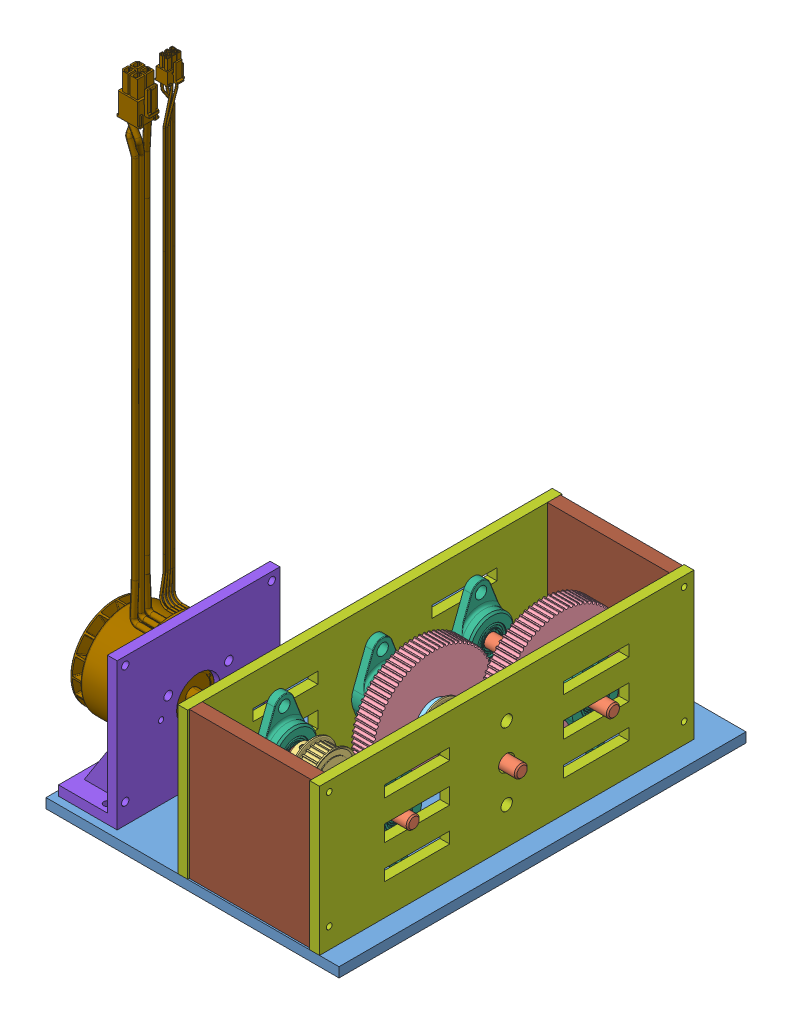
SolidWorks assembly Assembly, configuration Default. Lengths in mm.
Overall size (191.99 374.93 250).
22 component instances, 11 part files, 55 mates.
Components (placement in the parent):
- Base plate-1: Base plate [Default] at (107.5559 97.829 204.5167) size (180 6 250)
- 1265K67_Rotary Shaft-1: 1265K67_Rotary Shaft [1265K67] at (-105.0192 148.829 214.5167) x (0 -0.466171 -0.884694) z (1 0 0) size (8 8 100)
- 1265K67_Rotary Shaft-2: 1265K67_Rotary Shaft [1265K67] at (-110.9869 148.829 274.9267) x (0 -0.994866 -0.101198) z (1 0 0) size (8 8 100)
- 1265K67_Rotary Shaft-3: 1265K67_Rotary Shaft [1265K67] at (-108.8223 148.829 154.1067) x (0 0.698685 0.715429) z (1 0 0) size (8 8 100)
- 26toothpulley.stp-1: 26toothpulley.stp [Default] at (126.6866 148.829 274.9267) x (0 0.982193 0.187876) z (-1 0 0) size (28.1 28.1 20.6)
- 26toothpulley.stp-2: 26toothpulley.stp [Default] at (157.7866 148.829 214.5167) x (0 0.532948 0.846148) z (1 0 0) size (28.1 28.1 20.6)
- 80toothpulley.stp-1: 80toothpulley.stp [Default] at (146.2866 148.829 154.1067) x (0 0.075544 -0.997142) z (-1 0 0) size (75.56 75.56 22.2)
- 80toothpulley.stp-2: 80toothpulley.stp [Default] at (127.9866 148.829 214.5167) x (0 -0.170315 0.98539) z (-1 0 0) size (75.56 75.56 22.2)
- 94630A112_Steel Oversized Washer-1: 94630A112_Steel Oversized Washer [94630A112] at (144.9866 148.829 214.5167) x (0 -0.091283 0.995825) z (-1 0 0) size (23 23 4.3)
- 2820T42_Dry-Running Mounted Sleeve Bearing (1)-1: 2820T42_Dry-Running Mounted Sleeve Bearing (1) [2820T42] at (173.8059 148.829 154.1067) x (0 1 0) z (-1 0 0) size (57 28.5 11.75)
- 2820T42_Dry-Running Mounted Sleeve Bearing (1)-2: 2820T42_Dry-Running Mounted Sleeve Bearing (1) [2820T42] at (110.3059 148.829 274.9267) x (0 -1 0) z (1 0 0) size (57 28.5 11.75)
- 2820T42_Dry-Running Mounted Sleeve Bearing (1)-3: 2820T42_Dry-Running Mounted Sleeve Bearing (1) [2820T42] at (110.3059 148.829 214.5167) x (0 1 0) z (1 0 0) size (57 28.5 11.75)
- 2820T42_Dry-Running Mounted Sleeve Bearing (1)-4: 2820T42_Dry-Running Mounted Sleeve Bearing (1) [2820T42] at (173.8059 148.829 214.5167) x (0 1 0) z (-1 0 0) size (57 28.5 11.75)
- 2820T42_Dry-Running Mounted Sleeve Bearing (1)-5: 2820T42_Dry-Running Mounted Sleeve Bearing (1) [2820T42] at (110.3059 148.829 154.1067) x (0 -1 0) z (1 0 0) size (57 28.5 11.75)
- 2820T42_Dry-Running Mounted Sleeve Bearing (1)-6: 2820T42_Dry-Running Mounted Sleeve Bearing (1) [2820T42] at (173.8059 148.829 274.9267) x (0 1 0) z (-1 0 0) size (57 28.5 11.75)
- Shaft_and_Bearing_plate-1: Shaft_and_Bearing_plate [Default] at (104.5559 148.829 214.5167) x (0 0 1) z (0 -1 0) size (230 6 90)
- Shaft_and_Bearing_plate-2: Shaft_and_Bearing_plate [Default] at (179.5559 148.829 214.5167) x (0 0 -1) z (0 -1 0) size (230 6 90)
- motor_plate-1: motor_plate [Default] at (56.653 148.829 274.9267) x (0 0 -1) z (0 1 0) size (100 36 90)
- EC60fl-200W-V2.stp-1: EC60fl-200W-V2.stp [Default] at (73.753 148.829 274.9267) x (-1 0 0) z (0 0 1) size (68.19 353.93 60)
- 2463K28_Clamping Precision Flexible Shaft Coupling-1: 2463K28_Clamping Precision Flexible Shaft Coupling [2463K28] at (80.6759 148.829 274.9267) x (0 -0.924225 -0.381849) z (1 0 0) size (26.29 26.14 30)
- side_plate-1: side_plate [Default] at (142.0559 148.829 100.5167) x (1 0 0) z (0 -1 0) size (75 8 90)
- side_plate-2: side_plate [Default] at (142.0559 148.829 320.5167) x (1 0 0) z (0 -1 0) size (75 8 90)
Mates (geometry in assembly coordinates):
- Concentric1: concentric: cylinder of 1265K67_Rotary Shaft-2 through (189.0131 148.829 274.9267) axis (-1 0 0) radius 4; cylinder of 26toothpulley.stp-1 through (118.4966 148.829 274.9267) axis (1 0 0) radius 3
- Concentric2: concentric: cylinder of 1265K67_Rotary Shaft-1 through (194.9808 148.829 214.5167) axis (-1 0 0) radius 4; cylinder of 80toothpulley.stp-2 through (118.0116 148.829 214.5167) axis (1 0 0) radius 4
- Concentric3: concentric anti-aligned: cylinder of 1265K67_Rotary Shaft-1 through (194.9808 148.829 214.5167) axis (-1 0 0) radius 4; cylinder of 94630A112_Steel Oversized Washer-1 through (140.6866 148.829 214.5167) axis (1 0 0) radius 4.2
- Concentric4: concentric aligned: cylinder of 1265K67_Rotary Shaft-1 through (194.9808 148.829 214.5167) axis (-1 0 0) radius 4; cylinder of 26toothpulley.stp-2 through (165.9766 148.829 214.5167) axis (-1 0 0) radius 3
- Coincident2: coincident anti-aligned: plane of 80toothpulley.stp-2 through (140.6866 148.829 214.5167) normal (1 0 0); circle of 94630A112_Steel Oversized Washer-1
- Coincident3: coincident anti-aligned: plane of 26toothpulley.stp-2 through (144.9866 148.829 214.5167) normal (-1 0 0); plane of 94630A112_Steel Oversized Washer-1 through (144.9866 148.829 214.5167) normal (1 0 0)
- Concentric6: concentric anti-aligned: cylinder of 1265K67_Rotary Shaft-3 through (191.1777 148.829 154.1067) axis (-1 0 0) radius 4; cylinder of 80toothpulley.stp-1 through (136.3116 148.829 154.1067) axis (1 0 0) radius 4
- Concentric7: concentric: cylinder of 1265K67_Rotary Shaft-3 through (191.1777 148.829 154.1067) axis (-1 0 0) radius 4; cylinder of 2820T42_Dry-Running Mounted Sleeve Bearing (1)-1 through (168.0559 148.829 154.1067) axis (-1 0 0) radius 3.995
- Concentric8: concentric: cylinder of 1265K67_Rotary Shaft-3 through (191.1777 148.829 154.1067) axis (-1 0 0) radius 4; cylinder of 2820T42_Dry-Running Mounted Sleeve Bearing (1)-5 through (116.0559 148.829 154.1067) axis (1 0 0) radius 3.995
- Concentric9: concentric: cylinder of 1265K67_Rotary Shaft-1 through (194.9808 148.829 214.5167) axis (-1 0 0) radius 4; cylinder of 2820T42_Dry-Running Mounted Sleeve Bearing (1)-4 through (168.0559 148.829 214.5167) axis (-1 0 0) radius 3.995
- Concentric10: concentric anti-aligned: cylinder of 1265K67_Rotary Shaft-1 through (194.9808 148.829 214.5167) axis (-1 0 0) radius 4; cylinder of 2820T42_Dry-Running Mounted Sleeve Bearing (1)-3 through (116.0559 148.829 214.5167) axis (1 0 0) radius 3.995
- Concentric11: concentric: cylinder of 1265K67_Rotary Shaft-2 through (189.0131 148.829 274.9267) axis (-1 0 0) radius 4; cylinder of 2820T42_Dry-Running Mounted Sleeve Bearing (1)-6 through (168.0559 148.829 274.9267) axis (-1 0 0) radius 3.995
- Concentric12: concentric: cylinder of 1265K67_Rotary Shaft-2 through (189.0131 148.829 274.9267) axis (-1 0 0) radius 4; cylinder of 2820T42_Dry-Running Mounted Sleeve Bearing (1)-2 through (116.0559 148.829 274.9267) axis (1 0 0) radius 3.995
- Concentric13: concentric: cylinder of 1265K67_Rotary Shaft-1 through (194.9808 148.829 214.5167) axis (-1 0 0) radius 4; cylinder of Shaft_and_Bearing_plate-1 through (98.5559 148.829 214.5167) axis (1 0 0) radius 5
- Coincident4: coincident: plane of Base plate-1 through (107.5559 103.829 204.5167) normal (0 1 0); plane of Shaft_and_Bearing_plate-1 through (98.5559 103.829 99.5167) normal (0 -1 0)
- Coincident5: coincident: plane of Base plate-1 through (107.5559 103.829 204.5167) normal (0 1 0); plane of Shaft_and_Bearing_plate-2 through (185.5559 103.829 329.5167) normal (0 -1 0)
- Parallel1: parallel: line of Base plate-1 through (197.5559 103.829 329.5167) axis (0 0 -1); line of Shaft_and_Bearing_plate-2 through (197.5559 103.829 329.5167) axis (0 0 -1)
- Parallel2: parallel: line of Shaft_and_Bearing_plate-1 through (86.5559 103.829 99.5167) axis (0 0 1); line of Base plate-1 through (17.5559 103.829 79.5167) axis (0 0 1)
- Concentric14: concentric: cylinder of 1265K67_Rotary Shaft-1 through (194.9808 148.829 214.5167) axis (-1 0 0) radius 4; cylinder of Shaft_and_Bearing_plate-2 through (185.5559 148.829 214.5167) axis (-1 0 0) radius 5
- Concentric16: concentric: cylinder of 2820T42_Dry-Running Mounted Sleeve Bearing (1)-4 through (174.7559 171.079 214.5167) axis (1 0 0) radius 3.5; cylinder of Shaft_and_Bearing_plate-2 through (185.5559 171.079 214.5167) axis (-1 0 0) radius 3.5
- Coincident8: coincident anti-aligned: plane of 2820T42_Dry-Running Mounted Sleeve Bearing (1)-3 through (104.5559 126.579 214.5167) normal (-1 0 0); plane of Shaft_and_Bearing_plate-1 through (104.5559 148.829 214.5167) normal (1 0 0)
- Concentric18: concentric anti-aligned: cylinder of 2820T42_Dry-Running Mounted Sleeve Bearing (1)-3 through (109.3559 171.079 214.5167) axis (-1 0 0) radius 3.5; cylinder of Shaft_and_Bearing_plate-1 through (98.5559 171.079 214.5167) axis (1 0 0) radius 3.5
- Coincident9: coincident anti-aligned: plane of 2820T42_Dry-Running Mounted Sleeve Bearing (1)-4 through (179.5559 126.579 214.5167) normal (1 0 0); plane of Shaft_and_Bearing_plate-2 through (179.5559 148.829 214.5167) normal (-1 0 0)
- Tangent1: tangent anti-aligned: cylinder of 2820T42_Dry-Running Mounted Sleeve Bearing (1)-5 through (109.3559 171.079 154.1067) axis (-1 0 0) radius 3.5; plane of Shaft_and_Bearing_plate-1 through (98.5559 167.579 179.5167) normal (0 1 0)
- Tangent2: tangent: cylinder of 2820T42_Dry-Running Mounted Sleeve Bearing (1)-5 through (109.3559 126.579 154.1067) axis (-1 0 0) radius 3.5; plane of Shaft_and_Bearing_plate-1 through (98.5559 123.079 179.5167) normal (0 1 0)
- Coincident10: coincident anti-aligned: plane of 2820T42_Dry-Running Mounted Sleeve Bearing (1)-5 through (104.5559 171.079 154.1067) normal (-1 0 0); plane of Shaft_and_Bearing_plate-1 through (104.5559 148.829 214.5167) normal (1 0 0)
- Tangent3: tangent: cylinder of 2820T42_Dry-Running Mounted Sleeve Bearing (1)-1 through (174.7559 171.079 154.1067) axis (1 0 0) radius 3.5; plane of Shaft_and_Bearing_plate-2 through (185.5559 167.579 179.5167) normal (0 1 0)
- Tangent4: tangent: cylinder of 2820T42_Dry-Running Mounted Sleeve Bearing (1)-1 through (174.7559 126.579 154.1067) axis (1 0 0) radius 3.5; plane of Shaft_and_Bearing_plate-2 through (185.5559 123.079 179.5167) normal (0 1 0)
- Coincident11: coincident: plane of 2820T42_Dry-Running Mounted Sleeve Bearing (1)-1 through (179.5559 126.579 154.1067) normal (1 0 0); plane of Shaft_and_Bearing_plate-2 through (179.5559 148.829 214.5167) normal (-1 0 0)
- Coincident12: coincident: line of Base plate-1 through (197.5559 103.829 329.5167) axis (0 0 -1); line of Shaft_and_Bearing_plate-2 through (197.5559 103.829 329.5167) axis (0 0 -1)
- Tangent8: tangent: cylinder of 2820T42_Dry-Running Mounted Sleeve Bearing (1)-6 through (174.7559 171.079 274.9267) axis (1 0 0) radius 3.5; plane of Shaft_and_Bearing_plate-2 through (185.5559 167.579 249.5167) normal (0 1 0)
- Tangent9: tangent: cylinder of 2820T42_Dry-Running Mounted Sleeve Bearing (1)-6 through (174.7559 126.579 274.9267) axis (1 0 0) radius 3.5; plane of Shaft_and_Bearing_plate-2 through (185.5559 123.079 249.5167) normal (0 1 0)
- Coincident13: coincident: plane of 2820T42_Dry-Running Mounted Sleeve Bearing (1)-6 through (179.5559 126.579 274.9267) normal (1 0 0); plane of Shaft_and_Bearing_plate-2 through (179.5559 148.829 214.5167) normal (-1 0 0)
- Coincident14: coincident: line of Base plate-1 through (17.5559 103.829 329.5167) axis (1 0 0); line of Shaft_and_Bearing_plate-2 through (185.5559 103.829 329.5167) axis (-1 0 0)
- Tangent10: tangent: cylinder of 2820T42_Dry-Running Mounted Sleeve Bearing (1)-2 through (109.3559 171.079 274.9267) axis (-1 0 0) radius 3.5; plane of Shaft_and_Bearing_plate-1 through (98.5559 167.579 249.5167) normal (0 1 0)
- Tangent11: tangent: cylinder of 2820T42_Dry-Running Mounted Sleeve Bearing (1)-2 through (109.3559 126.579 274.9267) axis (-1 0 0) radius 3.5; plane of Shaft_and_Bearing_plate-1 through (98.5559 123.079 249.5167) normal (0 1 0)
- Coincident15: coincident anti-aligned: plane of 2820T42_Dry-Running Mounted Sleeve Bearing (1)-2 through (104.5559 171.079 274.9267) normal (-1 0 0); plane of Shaft_and_Bearing_plate-1 through (104.5559 148.829 214.5167) normal (1 0 0)
- Coincident17: coincident: plane of 26toothpulley.stp-1 through (127.9866 148.829 274.9267) normal (1 0 0); plane of 80toothpulley.stp-2 through (127.9866 148.829 214.5167) normal (-1 0 0)
- Coincident19: coincident anti-aligned: plane of 26toothpulley.stp-2 through (146.2866 148.829 214.5167) normal (1 0 0); plane of 80toothpulley.stp-1 through (146.2866 148.829 154.1067) normal (-1 0 0)
- Coincident20: coincident: plane of Base plate-1 through (107.5559 103.829 204.5167) normal (0 1 0); plane of motor_plate-1 through (50.653 103.829 224.9267) normal (0 -1 0)
- Concentric19: concentric anti-aligned: cylinder of motor_plate-1 through (50.653 148.829 274.9267) axis (1 0 0) radius 13.5; cylinder of EC60fl-200W-V2.stp-1 through (76.818 148.829 274.9267) axis (-1 0 0) radius 4
- Concentric20: concentric: cylinder of 1265K67_Rotary Shaft-2 through (189.0131 148.829 274.9267) axis (-1 0 0) radius 4; cylinder of motor_plate-1 through (50.653 148.829 274.9267) axis (1 0 0) radius 13.5
- Concentric22: concentric aligned: cylinder of motor_plate-1 through (50.653 159.579 293.5463) axis (1 0 0) radius 2.65; cylinder of EC60fl-200W-V2.stp-1 through (42.262 159.579 293.5463) axis (1 0 0) radius 1.65
- Coincident21: coincident anti-aligned: plane of motor_plate-1 through (50.653 148.829 274.9267) normal (-1 0 0); plane of EC60fl-200W-V2.stp-1 through (50.653 148.829 274.9267) normal (1 0 0)
- Coincident23: coincident: circle of 1265K67_Rotary Shaft-2; circle of 2463K28_Clamping Precision Flexible Shaft Coupling-1
- Coincident24: coincident: circle of EC60fl-200W-V2.stp-1; circle of 2463K28_Clamping Precision Flexible Shaft Coupling-1
- Distance2: distance = 60.41 mm: cylinder of 1265K67_Rotary Shaft-1 through (194.9808 148.829 214.5167) axis (-1 0 0) radius 4; cylinder of 1265K67_Rotary Shaft-2 through (189.0131 148.829 274.9267) axis (-1 0 0) radius 4
- Distance4: distance = 60.41 mm: cylinder of 1265K67_Rotary Shaft-3 through (191.1777 148.829 154.1067) axis (-1 0 0) radius 4; cylinder of 1265K67_Rotary Shaft-1 through (194.9808 148.829 214.5167) axis (-1 0 0) radius 4
- Coincident27: coincident: plane of Base plate-1 through (107.5559 103.829 204.5167) normal (0 1 0); plane of side_plate-2 through (104.5559 103.829 328.5167) normal (0 -1 0)
- Coincident28: coincident: plane of Base plate-1 through (107.5559 103.829 204.5167) normal (0 1 0); plane of side_plate-1 through (104.5559 103.829 108.5167) normal (0 -1 0)
- Concentric27: concentric: circle of Shaft_and_Bearing_plate-1; circle of side_plate-2
- Coincident29: coincident anti-aligned: plane of Shaft_and_Bearing_plate-1 through (104.5559 148.829 214.5167) normal (1 0 0); plane of side_plate-2 through (104.5559 193.829 328.5167) normal (-1 0 0)
- Concentric28: concentric: circle of Shaft_and_Bearing_plate-2; circle of side_plate-1
- Coincident30: coincident: plane of Shaft_and_Bearing_plate-1 through (104.5559 148.829 214.5167) normal (1 0 0); plane of side_plate-1 through (104.5559 193.829 108.5167) normal (-1 0 0)
- Coincident31: coincident: plane of Shaft_and_Bearing_plate-2 through (179.5559 148.829 214.5167) normal (-1 0 0); plane of side_plate-1 through (179.5559 193.829 108.5167) normal (1 0 0)
